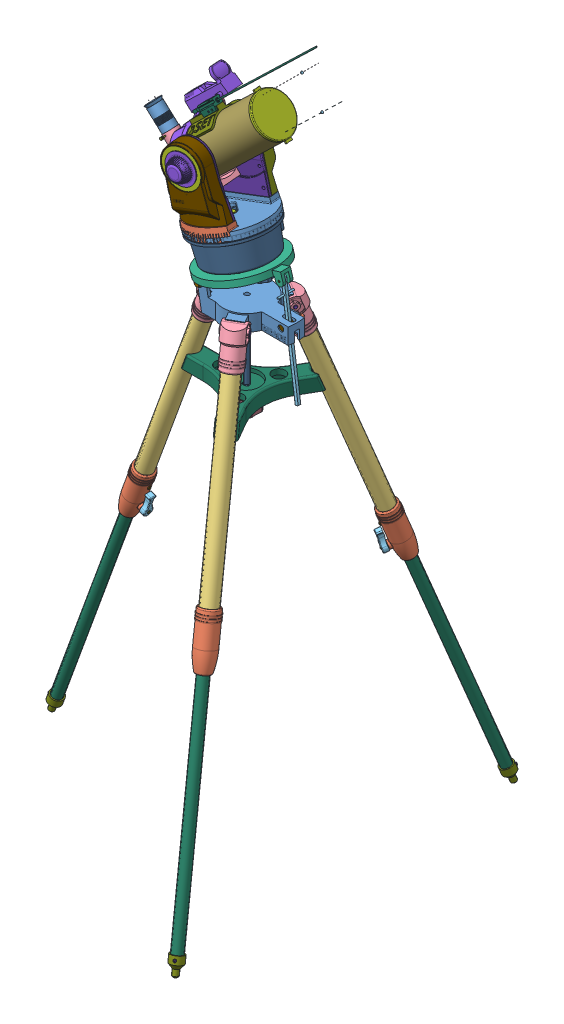
SolidWorks assembly telescope assemblage, configuration Défaut. Lengths in mm.
Overall size (798.62 1786.17 885.88).
260 component instances, 126 part files, 44 mates.
Components (placement in the parent):
- plateforme trepied-1: plateforme trepied [Défaut] at (-10.3731 0 -20) x (0 0 1) z (0 1 0) size (184.28 220 78.5)
- tube superieur-1: tube superieur [Défaut] at (-282.0109 -548.273 -53.7859) x (0 0 -1) z (-0.939693 0.34202 0) size (56 647 70.31)
  - liaison tube-1: liaison tube [Défaut] at (-33.7859 -53.3876 0) size (49 123 52)
  - tube superieur-1: tube superieur [Défaut] at (-33.7859 -3.3876 0) x (1 0 0) z (0 -1 0) size (38 38 530)
  - liaison tube plaque-1: liaison tube plaque [Défaut] at (-33.7859 -483.3876 0) x (-1 0 0) z (0 0 1) size (54 94 52.5)
  - manette fixation pied-1: manette fixation pied [Défaut] at (-52.9516 19.4533 -40.9) x (-1 0 0) z (0 0 1) size (22 50 29.31)
    - manette fixation pied-1: manette fixation pied [Défaut] at (-19.1657 -10.1591 0) size (22 50 15.3)
    - vis M8 fixation pied-1: vis M8 fixation pied [Défaut] at (-19.1657 -10.1591 6.2) x (1 0 0) z (0 -1 0) size (11 21.7 11)
    - Vis cr f90 M4-1: Vis cr f90 M4 [Défaut] at (-19.1657 -10.1591 1.7) size (7.4 7.4 13.11)
  - VisChcM8 50-2: VisChcM8 50 [Défaut] at (-55.5859 -557.3876 0) x (0 0 -1) z (1 0 0) size (12.3 12.3 56)
  - Vis cr M5-1: Vis cr M5 [Défaut] at (-33.7859 -20.3876 -23.15) x (0 1 0) z (0 0 1) size (7.7 7.7 9.33)
  - Vis cr M5-2: Vis cr M5 [Défaut] at (-33.7859 -516.3876 -23.15) size (7.7 7.7 9.33)
- axe M12-1: axe M12 [Défaut] at (-10.3731 0 -20) x (-0.923728 0 0.383049) z (0 -1 0) size (12.15 12.3 255.78)
- rondelle 30-1: rondelle 30 [Défaut] at (-10.3731 -220.4136 -20) x (0.988696 0 0.149935) z (0 1 0) size (30 30 2.3)
- Ecrou hexagonal ISO 4032, M 12-1: Ecrou hexagonal ISO 4032, M 12 [Défaut] at (-10.3731 -29.8 -20) x (0.866025 0 0.5) z (-0.5 0 0.866025) size (20.78 10.8 18)
- ecrou plastic M12-1: ecrou plastic M12 [Défaut] at (-21.7775 -251.8636 -36.5397) x (-0.587785 0 -0.809017) z (0 1 0) size (58 55.29 30.73)
  - ecrou plastic-1: ecrou plastic [Défaut] at (-20.0843 0.4954 0) size (58 55.29 30)
  - insert M12-1: insert M12 [Défaut] at (-20.0843 0.4954 14.3) size (16 16 17.46)
- pied-1: pied [Défaut] at (-281.8601 -547.9154 -17.129) x (0 0 1) z (-0.34202 -0.939693 0) size (30.8 33.14 626.85)
  - tube inferieur-1: tube inferieur [Défaut] at (-2.871 0.0194 0) size (25 25 600)
  - pied-1: pied [Défaut] at (-2.871 0.0194 582.85) x (1 0 0) z (0 -1 0) size (30.8 44 30.8)
  - Vis cr M4-1: Vis cr M4 [Défaut] at (-2.871 15.3194 591.85) x (0 0 -1) z (0 -1 0) size (6.7 6.7 12.44)
- pied-2: pied [Défaut] at (122.8841 -547.9154 -256.5501) x (-0.866025 0 -0.5) z (0.17101 -0.939693 -0.296198) size (30.8 33.14 626.85)
  - tube inferieur-1: tube inferieur [Défaut] at (-2.871 0.0194 0) size (25 25 600)
  - pied-1: pied [Défaut] at (-2.871 0.0194 582.85) x (1 0 0) z (0 -1 0) size (30.8 44 30.8)
  - Vis cr M4-1: Vis cr M4 [Défaut] at (-2.871 15.3194 591.85) x (0 0 -1) z (0 -1 0) size (6.7 6.7 12.44)
- pied-3: pied [Défaut] at (127.8567 -547.9154 213.6791) x (0.866025 0 -0.5) z (0.17101 -0.939693 0.296198) size (30.8 33.14 626.85)
  - tube inferieur-1: tube inferieur [Défaut] at (-2.871 0.0194 0) size (25 25 600)
  - pied-1: pied [Défaut] at (-2.871 0.0194 582.85) x (1 0 0) z (0 -1 0) size (30.8 44 30.8)
  - Vis cr M4-1: Vis cr M4 [Défaut] at (-2.871 15.3194 591.85) x (0 0 -1) z (0 -1 0) size (6.7 6.7 12.44)
- tube superieur-2: tube superieur [Défaut] at (154.7052 -548.273 -238.3523) x (0.866025 0 0.5) z (0.469846 0.34202 -0.813798) size (56 647 70.31)
  - liaison tube-1: liaison tube [Défaut] at (-33.7859 -53.3876 0) size (49 123 52)
  - tube superieur-1: tube superieur [Défaut] at (-33.7859 -3.3876 0) x (1 0 0) z (0 -1 0) size (38 38 530)
  - liaison tube plaque-1: liaison tube plaque [Défaut] at (-33.7859 -483.3876 0) x (-1 0 0) z (0 0 1) size (54 94 52.5)
  - manette fixation pied-1: manette fixation pied [Défaut] at (-52.9516 19.4533 -40.9) x (-1 0 0) z (0 0 1) size (22 50 29.31)
    - manette fixation pied-1: manette fixation pied [Défaut] at (-19.1657 -10.1591 0) size (22 50 15.3)
    - vis M8 fixation pied-1: vis M8 fixation pied [Défaut] at (-19.1657 -10.1591 6.2) x (1 0 0) z (0 -1 0) size (11 21.7 11)
    - Vis cr f90 M4-1: Vis cr f90 M4 [Défaut] at (-19.1657 -10.1591 1.7) size (7.4 7.4 13.11)
  - VisChcM8 50-2: VisChcM8 50 [Défaut] at (-55.5859 -557.3876 0) x (0 0 -1) z (1 0 0) size (12.3 12.3 56)
  - Vis cr M5-1: Vis cr M5 [Défaut] at (-33.7859 -20.3876 -23.15) x (0 1 0) z (0 0 1) size (7.7 7.7 9.33)
  - Vis cr M5-2: Vis cr M5 [Défaut] at (-33.7859 -516.3876 -23.15) size (7.7 7.7 9.33)
- tube superieur-3: tube superieur [Défaut] at (96.1863 -548.273 232.1382) x (-0.866025 0 0.5) z (0.469846 0.34202 0.813798) size (56 647 70.31)
  - liaison tube-1: liaison tube [Défaut] at (-33.7859 -53.3876 0) size (49 123 52)
  - tube superieur-1: tube superieur [Défaut] at (-33.7859 -3.3876 0) x (1 0 0) z (0 -1 0) size (38 38 530)
  - liaison tube plaque-1: liaison tube plaque [Défaut] at (-33.7859 -483.3876 0) x (-1 0 0) z (0 0 1) size (54 94 52.5)
  - manette fixation pied-1: manette fixation pied [Défaut] at (-52.9516 19.4533 -40.9) x (-1 0 0) z (0 0 1) size (22 50 29.31)
    - manette fixation pied-1: manette fixation pied [Défaut] at (-19.1657 -10.1591 0) size (22 50 15.3)
    - vis M8 fixation pied-1: vis M8 fixation pied [Défaut] at (-19.1657 -10.1591 6.2) x (1 0 0) z (0 -1 0) size (11 21.7 11)
    - Vis cr f90 M4-1: Vis cr f90 M4 [Défaut] at (-19.1657 -10.1591 1.7) size (7.4 7.4 13.11)
  - VisChcM8 50-2: VisChcM8 50 [Défaut] at (-55.5859 -557.3876 0) x (0 0 -1) z (1 0 0) size (12.3 12.3 56)
  - Vis cr M5-1: Vis cr M5 [Défaut] at (-33.7859 -20.3876 -23.15) x (0 1 0) z (0 0 1) size (7.7 7.7 9.33)
  - Vis cr M5-2: Vis cr M5 [Défaut] at (-33.7859 -516.3876 -23.15) size (7.7 7.7 9.33)
- axe reglage altitude-1: axe reglage altitude [Défaut] at (94.0034 -12 -20) x (0.990738 0.135788 0) z (0 0 -1) size (14 14 35)
- VisM8 15 reglage montage equatorial-1: VisM8 15 reglage montage equatorial [Défaut] at (69.6004 -12.4568 -44.1703) x (-0.999825 -0.018716 0) z (0.018716 -0.999825 0) size (48.14 28.09 16.29)
  - languette-1: languette [Défaut] at (-24.4073 4.8297 0) size (45 10 2.8)
  - VisM8 15 reglage montage equatorial-1: VisM8 15 reglage montage equatorial [Défaut] at (-24.4073 -3.1703 0) x (0 0 1) z (0 -1 0) size (12 12 28.09)
  - CHCM3-10-1: CHCM3-10 [Défaut] at (-24.4073 4.8297 6.5) x (-1 0 0) z (0 0 -1) size (5 5 12.5)
  - rondelle 16-1: rondelle 16 [Défaut] at (-24.4073 -3.1703 0) x (0.999837 0 -0.018032) z (0 -1 0) size (16 16 1)
- regle-1: regle [Défaut] at (116.2056 -173.9924 -20) x (0 0 1) z (-0.135788 0.990738 0) size (40 8.8 260)
- plateau inclinable-1: plateau inclinable [Défaut] at (2.5363 78.221 -20) x (0.956126 0.292954 0) z (0.292954 -0.956126 0) size (206.4 185 50.37)
  - plateau inclinable-1: plateau inclinable [Défaut] at (-28.5 -0.1435 0) size (206.4 185 37.6)
  - Vis  M6-24-1: Vis  M6-24 [Défaut] at (75.7 -11.9435 22.75) x (-1 0 0) z (0 1 0) size (6 6 24)
  - rondelle 16-7: rondelle 16 [Défaut] at (-81.5 62.9965 28.6) x (-0.476926 0 0.878943) z (0 1 0) size (16 16 1)
  - rondelle 16-8: rondelle 16 [Défaut] at (-81.5 48 28.6) x (-0.476926 0 0.878943) z (0 1 0) size (16 16 1)
  - rondelle 16-9: rondelle 16 [Défaut] at (-81.5 56 28.6) x (-0.476926 0 0.878943) z (0 1 0) size (16 16 1)
  - rondelle 16-10: rondelle 16 [Défaut] at (-81.5 -56.2835 28.6) x (0.476926 0 -0.878943) z (0 -1 0) size (16 16 1)
  - rondelle 16-11: rondelle 16 [Défaut] at (-81.5 -48 28.6) x (0.476926 0 -0.878943) z (0 -1 0) size (16 16 1)
  - rondelle 16-12: rondelle 16 [Défaut] at (-81.5 -63.2835 28.6) x (0.476926 0 -0.878943) z (0 -1 0) size (16 16 1)
  - EcrouH8 nylstop-1: EcrouH8 nylstop [Défaut] at (-81.5 -48 28.6) x (0 0 -1) z (0 -1 0) size (13 15.01 7.1)
  - EcrouH8 nylstop-2: EcrouH8 nylstop [Défaut] at (-81.5 48 28.6) x (0 0 1) z (0 1 0) size (13 15.01 7.1)
  - VisHm8_25-1: VisHm8_25 [Défaut] at (-81.5 -64.2835 28.6) x (0.866025 0 0.5) z (0 1 0) size (13 15.01 29.5)
  - VisHm8_25-2: VisHm8_25 [Défaut] at (-81.5 63.9965 28.6) x (-0.866025 0 -0.5) z (0 -1 0) size (13 15.01 29.5)
  - vis plastique M6-1: vis plastique M6 [Défaut] at (-89.0406 -5.4634 33.1) x (-0.885007 -0.465577 0) z (0 0 -1) size (33.9 32.72 44.02)
    - bouton plastic-1: bouton plastic [Défaut] at (-10.2565 0.6155 0) size (33.9 32.72 15)
    - Vis  M6 30-1: Vis  M6 30 [Défaut] at (-10.2565 0.6155 15) x (-0.5 0.866025 0) z (0 0 1) size (10 11.55 34.02)
    - rondelle 12-1: rondelle 12 [Défaut] at (-10.2565 0.6155 32.1) size (11.9 11.9 1)
    - Truac-1: Truac [Défaut] at (-10.2565 0.6155 33.1) x (0 0 1) z (-0.309017 0.951057 0) size (0.6 8.54 9)
    - Ressort de compression, 9x0,4-1: Ressort de compression, 9x0,4 [Défaut] at (-10.2565 0.6155 32.1) x (0 0 -1) z (0.885007 0.465577 0) size (11.52 9.7 9.88)
  - vis plastique M6-2: vis plastique M6 [Défaut] at (14.4594 -5.4634 33.1) x (-0.885007 -0.465577 0) z (0 0 -1) size (33.9 32.72 44.02)
    - bouton plastic-1: bouton plastic [Défaut] at (-10.2565 0.6155 0) size (33.9 32.72 15)
    - Vis  M6 30-1: Vis  M6 30 [Défaut] at (-10.2565 0.6155 15) x (-0.5 0.866025 0) z (0 0 1) size (10 11.55 34.02)
    - rondelle 12-1: rondelle 12 [Défaut] at (-10.2565 0.6155 32.1) size (11.9 11.9 1)
    - Truac-1: Truac [Défaut] at (-10.2565 0.6155 33.1) x (0 0 1) z (-0.309017 0.951057 0) size (0.6 8.54 9)
    - Ressort de compression, 9x0,4-1: Ressort de compression, 9x0,4 [Défaut] at (-10.2565 0.6155 32.1) x (0 0 -1) z (0.885007 0.465577 0) size (11.52 9.7 9.88)
- cale-1: cale [Défaut] at (-13.285 -219.2636 -20) x (0 0 1) z (0 1 0) size (261.88 228.05 35)
- meade-1: meade [Défaut] at (-48.2669 146.7444 -20.1435) x (-0.956126 -0.292954 0) z (0 0 -1) size (480.47 493.64 231.58)
  - fourche-1: fourche [Défaut] at (-637.6539 13.0791 484.13) x (0.045417 -0.017413 0.998816) z (-0.998966 0.001172 0.045444) size (198.85 238.33 188.61)
    - branche equilibrage-1: branche equilibrage [Défaut] at (-444.0293 45.9192 -837.0232) x (0.999848 0.017413 0.00001) z (0.00001 -0.001172 0.999999) size (42.16 177.75 110.07)
    - Plaque carter équilibrage-1: Plaque carter équilibrage [Défaut] at (-443.0317 45.9366 -837.0903) x (0.999848 0.017413 0.00001) z (0.00001 -0.001172 0.999999) size (27.56 165.18 109.18)
    - Plaque carter équilibrage-2: Plaque carter équilibrage [Défaut] at (-468.0617 45.0668 -480.7137) x (-0.999848 -0.017413 -0.00001) z (-0.00001 0.001172 -0.999999) size (27.56 165.18 109.18)
    - branche motorisée-1: branche motorisée [Défaut] at (-441.716 45.9434 -837.1795) x (0.999848 0.017413 0.00001) z (0.00001 -0.001172 0.999999) size (49.59 177.72 110.04)
    - PIED DE fourche-1: PIED DE fourche [Défaut] at (-454.4692 -14.4541 -658.8869) x (0.999848 0.017413 0.00001) z (0.00001 -0.001172 0.999999) size (191.94 35.1 188.57)
      - Pied de fourche-1: Pied de fourche [Défaut] at (12.1809 59.9857 -178.2534) size (191.94 35.1 188.57)
      - Pied de fourche1-1: Pied de fourche1 [Défaut] at (-12.1809 59.9857 178.0188) x (-1 0 0) z (0 0 -1) size (54.8 35.1 115.86)
    - rondelle vis m8_50-1: rondelle vis m8_50 [Défaut] at (-454.2843 -25.0712 -659.0167) x (0.997592 0.017452 -0.067129) z (0.017413 -0.999848 -0.001172) size (26.8 26.16 7)
    - VisHM8_50-1: VisHM8_50 [Défaut] at (-454.3818 -19.4721 -659.0102) x (0.997592 0.017452 -0.067129) z (0.017413 -0.999848 -0.001172) size (12.6 14.55 55.47)
    - limiteur de couple embase-1: limiteur de couple embase [Défaut] at (-453.5008 -70.0544 -659.0694) x (0.06714 0 0.997744) z (-0.997592 -0.017452 0.067129) size (25.3 5 25.3)
    - Roue à denture hélicoïdale m=0,5 Z=60-1: Roue à denture hélicoïdale m=0,5 Z=60 [Défaut] at (-453.6431 -61.8856 -659.0599) x (0.201032 0.002353 0.979582) z (-0.017413 0.999848 0.001172) size (31.07 31.07 6.34)
    - Levier de débrayage-1: Levier de débrayage [Défaut] at (-491.4971 43.1006 -833.8173) x (0.963244 0.01709 -0.268082) z (0.268062 0.003539 0.963395) size (36.12 10 38.96)
    - plateau-1: plateau [Défaut] at (-454.3861 -19.2221 -659.0099) x (-0.997592 -0.017452 0.067129) z (0.017413 -0.999848 -0.001172) size (170 170 47)
    - EcrouHM 20-2: EcrouHM 20 [Défaut] at (-453.9456 -44.5183 -659.0395) x (0.06714 0 0.997744) z (-0.017413 0.999848 0.001172) size (30 34.64 12)
    - motoreducteur fourche-1: motoreducteur fourche [Défaut] at (-542.1299 45.8782 -641.824) x (0.06714 0 0.997744) z (0.997592 0.017452 -0.067129) size (70.5 139.71 33.06)
      - rep. 01 pignon arbre moteur + disque-1: rep. 01 pignon arbre moteur + disque [Défaut] at (0 -0.36 0) size (19 10.8 19)
      - rep. 02-03 roue Z56-1: rep. 02-03 roue Z56 [Défaut] at (0.8779 -0.6486 0.8082) x (0.995701 0 0.092628) z (-0.092628 0 0.995701) size (28.76 10.95 28.76)
      - rep. 08-09 roue inter-1: rep. 08-09 roue inter [Défaut] at (-0.15 -0.2381 0) x (1 0 0) z (0 0 1) size (12.96 5.74 12.96)
      - rep. 06-07 roue inter-1: rep. 06-07 roue inter [Défaut] at (-0.15 -0.0981 0) x (1 0 0) z (0 0 1) size (13 5.74 13)
      - rep. 04-05 roue inter-1: rep. 04-05 roue inter [Défaut] at (-21.6079 -0.6386 5.1059) x (0.907401 0 -0.420265) z (0.420265 0 0.907401) size (13 5.74 13)
      - bati-1: bati [Défaut] at (103.3128 129.885 -87.3106) size (70.5 138.91 24)
        - Axe Rep19bis-1: Axe Rep19bis [Défaut] at (-92.1856 -130.245 98.2871) x (-0.137137 0 0.990552) z (-0.990552 0 -0.137137) size (3 14 3)
        - moteur-1: moteur [Défaut] at (-103.3128 -129.885 87.3106) size (18 46.5 24)
        - axe-1: axe [Défaut] at (-111.605 -120.0821 97.7106) x (0.934599 0 -0.355704) z (0 -1 0) size (3 3 39)
        - bati2-1: bati2 [Défaut] at (-77.4849 -277.8736 138.6581) x (1 0 0) z (0 0 -1) size (17.4 55.11 17.4)
          - rondelle alu-1: rondelle alu [Défaut] at (-55.9783 -35.2009 30.6529) size (17.4 2.5 17.4)
          - Rondelle M6_1-1: Rondelle M6_1 [Défaut] at (-55.9783 -35.2009 30.6529) size (16.67 2.55 16.67)
          - rondelle alu_1-1: rondelle alu_1 [Défaut] at (-55.9783 -35.2009 30.6529) size (17.4 2.5 17.4)
          - Entretoise_1-1: Entretoise_1 [Défaut] at (-55.9783 -35.2009 30.6529) size (16.5 6 16.5)
          - Entretoise-1: Entretoise [Défaut] at (-55.9783 -35.2009 30.6529) size (16.5 6 16.5)
          - Rondelle M6-1: Rondelle M6 [Défaut] at (-55.9783 -35.2009 30.6529) size (16.67 2.55 16.67)
          - rep. 16 Ecrou M6-1: rep. 16 Ecrou M6 [Défaut] at (18.5294 -120.4752 48.0628) x (-0.896454 0 -0.443136) z (-0.443136 0 0.896454) size (12.68 6 11.39)
        - corps1-1: corps1 [Défaut] at (-126.5989 -147.7633 97.7106) size (62.7 74.5 12)
        - corps2-1: corps2 [Défaut] at (-126.5989 -147.7633 85.7106) size (62.7 50 12) (hidden)
        - châpe en alu-1: châpe en alu [Défaut] at (-133.4632 -157.3984 87.2051) size (33.3 38 19.61)
      - vis-1: vis [Défaut] at (7.3554 -71.4832 9.6533) x (1 0 0) z (0 1 0) size (33.09 33.06 82.71)
        - Vis san fin m=0,5 - 1 filet(s)-2: Vis san fin m=0,5 - 1 filet(s) [Défaut] at (-0.6479 -0.6412 0.3804) x (0.7262 -0.687484 0) z (0 0 1) size (8.16 8.16 68.9)
        - rep12-4: rep12 [Défaut] at (-11.6724 36.0347 43.7266) x (0.537117 -0.843508 0) z (-0.843508 -0.537117 0) size (23.91 29.81 24)
      - engrenage-1: engrenage [Défaut] at (-45.9983 -125.8694 31.0757) x (-0.919401 0 0.393321) z (0.393321 0 0.919401) size (12.99 17.44 12.99)
        - rep.11SLDPRT-1: rep.11SLDPRT [Défaut] at (-64.557 -106.8565 -14.5787) size (9.52 16 9.52)
        - rep. yacine-1: rep. yacine [Défaut] at (-64.557 -106.8565 -14.5787) size (12.99 1.44 12.99)
      - Vis à tête cylindrique à six pans creux Chc M2,5 - 8-1: Vis à tête cylindrique à six pans creux Chc M2,5 - 8 [Défaut] at (6.7074 -20.6971 10.2945) x (0.636786 0 0.771041) z (0 -1 0) size (4.2 4.2 10.57)
      - joint 9 5 emb-1: joint 9 5 emb [Défaut] at (6.7074 -89.1506 10.2945) size (13.5 2 13.5)
      - joint 9 5 emb-2: joint 9 5 emb [Défaut] at (6.7074 -53.1506 10.2945) size (13.5 2 13.5)
    - Vis sans tête à six pans creux à bout cuvette M3 - 3-1: Vis sans tête à six pans creux à bout cuvette M3 - 3 [Réaliste] at (-445.1418 -17.1499 -659.6319) x (-0.019293 -0.859815 -0.51024) z (0.066624 -0.510307 0.857408) size (3.03 3.08 3.04)
    - Vis à tête cylindrique bombée cruciforme type H M3 - 10-1: Vis à tête cylindrique bombée cruciforme type H M3 - 10 [Filetage Réaliste] at (-521.841 56.7793 -695.504) x (-0.997592 -0.017452 0.067129) z (-0.0364 0.955572 -0.292501) size (12.58 5.6 5.6)
    - Vis à tête cylindrique bombée cruciforme type H M3 - 10-2: Vis à tête cylindrique bombée cruciforme type H M3 - 10 [Filetage Réaliste] at (-508.9533 16.8988 -611.179) x (-0.997592 -0.017452 0.067129) z (-0.040277 -0.642181 -0.765494) size (12.58 5.6 5.6)
    - Vis à tête cylindrique bombée cruciforme type H M3 - 10-3: Vis à tête cylindrique bombée cruciforme type H M3 - 10 [Filetage Réaliste] at (-514.8616 16.8988 -698.9804) x (-0.997592 -0.017452 0.067129) z (-0.068087 0.06176 -0.995766) size (12.58 5.6 5.6)
    - Vis à tête cylindrique bombée cruciforme type H M3 - 10-4: Vis à tête cylindrique bombée cruciforme type H M3 - 10 [Filetage Réaliste] at (-521.2936 154.7556 -654.4481) x (-0.997592 -0.017452 0.067129) z (-0.06714 0 -0.997744) size (12.58 5.6 5.6)
    - Vis à tête cylindrique bombée cruciforme type H M3 - 10-5: Vis à tête cylindrique bombée cruciforme type H M3 - 10 [Filetage Réaliste] at (-516.3356 56.7793 -613.689) x (-0.997592 -0.017452 0.067129) z (-0.06714 0 -0.997744) size (12.58 5.6 5.6)
    - Vis à tête cylindrique bombée cruciforme type H M3 - 10-7: Vis à tête cylindrique bombée cruciforme type H M3 - 10 [Filetage Réaliste] at (-393.6444 157.0051 -663.0973) x (0.997592 0.017452 -0.067129) z (0.06714 0 0.997744) size (12.58 5.6 5.6)
    - Vis à tête cylindrique bombée cruciforme type H M3 - 10-8: Vis à tête cylindrique bombée cruciforme type H M3 - 10 [Filetage Réaliste] at (-401.1787 18.9039 -706.6898) x (0.997592 0.017452 -0.067129) z (0.06714 0 0.997744) size (12.58 5.6 5.6)
    - Vis à tête cylindrique bombée cruciforme type H M3 - 10-10: Vis à tête cylindrique bombée cruciforme type H M3 - 10 [Filetage Réaliste] at (-395.1895 59.0113 -704.086) x (0.997592 0.017452 -0.067129) z (0.06714 0 0.997744) size (12.58 5.6 5.6)
    - Vis à tête cylindrique fendue CS M4 - 10-1: Vis à tête cylindrique fendue CS M4 - 10 [Défaut] at (-539.7157 125.5672 -628.3483) x (0.067415 -0.016315 0.997592) z (-0.997592 -0.017452 0.067129) size (7 7 10.62)
    - Vis à tête cylindrique fendue CS M4 - 10-2: Vis à tête cylindrique fendue CS M4 - 10 [Défaut] at (-538.2089 116.0774 -615.8713) x (0.067415 -0.016315 0.997592) z (-0.997592 -0.017452 0.067129) size (7 7 10.62)
    - Vis à tête cylindrique fendue CS M4 - 10-3: Vis à tête cylindrique fendue CS M4 - 10 [Défaut] at (-539.3849 106.5701 -628.3705) x (0.067415 -0.016315 0.997592) z (-0.997592 -0.017452 0.067129) size (7 7 10.62)
    - Vis à tête cylindrique bombée cruciforme type H M3 - 12-2: Vis à tête cylindrique bombée cruciforme type H M3 - 12 [Filetage Réaliste] at (-395.2704 18.9039 -618.8883) x (0.997592 0.017452 -0.067129) z (0.067129 0.000586 0.997744) size (14.59 5.6 5.6)
    - Vis à tête cylindrique bombée cruciforme type H M3 - 12-3: Vis à tête cylindrique bombée cruciforme type H M3 - 12 [Filetage Réaliste] at (-389.684 59.0113 -622.271) x (0.997592 0.017452 -0.067129) z (0.068185 -0.42423 0.902984) size (14.59 5.6 5.6)
    - Vis à tête cylindrique bombée cruciforme type H M3 - 25-1: Vis à tête cylindrique bombée cruciforme type H M3 - 25 [Filetage Réaliste] at (-516.5693 58.6063 -628.1014) x (-0.997592 -0.017452 0.067129) z (-0.067129 0.486457 -0.871122) size (32.61 5.6 5.6)
    - Vis à tête cylindrique bombée cruciforme type H M3 - 25-2: Vis à tête cylindrique bombée cruciforme type H M3 - 25 [Filetage Réaliste] at (-520.3322 72.7741 -680.3366) x (-0.997592 -0.017452 0.067129) z (-0.067129 0.486457 -0.871122) size (32.61 5.6 5.6)
    - Vis à tête cylindrique bombée cruciforme type H M3 - 25-3: Vis à tête cylindrique bombée cruciforme type H M3 - 25 [Filetage Réaliste] at (-519.8272 43.7786 -680.3706) x (-0.997592 -0.017452 0.067129) z (0.067053 0.00493 0.997737) size (32.61 5.6 5.6)
    - Vis à tête cylindrique bombée cruciforme type H M3 - 20-1: Vis à tête cylindrique bombée cruciforme type H M3 - 20 [Filetage Réaliste] at (-531.1265 -25.9655 -653.8459) x (-0.017413 0.999848 0.001172) z (0.998816 0.017342 0.045444) size (22.61 5.6 5.6)
    - Vis à tête cylindrique bombée cruciforme type H M3 - 20-2: Vis à tête cylindrique bombée cruciforme type H M3 - 20 [Filetage Réaliste] at (-512.8439 -25.695 -612.9812) x (-0.017413 0.999848 0.001172) z (0.998816 0.017342 0.045444) size (22.61 5.6 5.6)
    - Vis à tête cylindrique bombée cruciforme type H M3 - 20-3: Vis à tête cylindrique bombée cruciforme type H M3 - 20 [Filetage Réaliste] at (-517.7505 -25.6821 -696.841) x (-0.017413 0.999848 0.001172) z (0.998816 0.017342 0.045444) size (22.61 5.6 5.6)
    - Vis à tête cylindrique bombée cruciforme type H M3 - 20-4: Vis à tête cylindrique bombée cruciforme type H M3 - 20 [Filetage Réaliste] at (-395.7403 -23.5476 -705.0512) x (-0.017413 0.999848 0.001172) z (0.998816 0.017342 0.045444) size (22.61 5.6 5.6)
    - Vis à tête cylindrique bombée cruciforme type H M3 - 20-5: Vis à tête cylindrique bombée cruciforme type H M3 - 20 [Filetage Réaliste] at (-377.4577 -23.2771 -664.1865) x (-0.017413 0.999848 0.001172) z (0.998816 0.017342 0.045444) size (22.61 5.6 5.6)
    - Vis à tête cylindrique bombée cruciforme type H M3 - 20-6: Vis à tête cylindrique bombée cruciforme type H M3 - 20 [Filetage Réaliste] at (-390.8337 -23.5604 -621.1914) x (-0.017413 0.999848 0.001172) z (0.998816 0.017342 0.045444) size (22.61 5.6 5.6)
  - tube-1: tube [Défaut] at (-30.0954 77.7985 3.4044) x (0.112402 0 0.993663) z (-0.888013 0.448711 0.100451) size (229.47 195.18 484.9)
    - Capuchon port photo-2: Capuchon port photo [Défaut] at (20.0265 52.1414 -183.8549) x (0.753442 -0.654583 0.06202) z (-0.29492 -0.252137 0.921656) size (39.95 39.82 23.78)
    - support objectif-2: support objectif [Défaut] at (0 67.5 -76) size (179.88 130.77 134.7)
    - Palier d'embrayage-2: Palier d'embrayage [Défaut] at (24.7034 252.6163 -72.3954) x (0.997744 -0.06714 0) z (-0.06714 -0.997744 0) size (14.91 34.8 28.76)
    - palier-2: palier [Défaut] at (-93.6662 67.5 0) x (1 0 0) z (0 -0.589029 0.808112) size (10.05 25.5 25.5)
    - Roue à denture hélicoïdale m=0,5 Z=60-3: Roue à denture hélicoïdale m=0,5 Z=60 [Défaut] at (-77.15 67.5 0) x (0 0.783284 -0.621664) z (1 0 0) size (31.07 31.07 6.34)
    - Plaque repérage angulaire-3: Plaque repérage angulaire [Défaut] at (-159.1429 162.8547 -174.0321) x (0.997744 -0.051519 0.043053) z (-0.06714 -0.765605 0.639798) size (6.77 89 88.85)
    - molette blocage vertical-2: molette blocage vertical [Défaut] at (25.2373 156.4775 -169.1848) x (0.997744 -0.051429 0.043161) z (-0.06714 -0.764265 0.641398) size (31.87 70 69.98)
    - molette blocage 2 vertical-2: molette blocage 2 vertical [Défaut] at (-32.8172 155.1442 169.8822) x (-0.997741 -0.051084 -0.043619) z (0.067172 -0.759198 -0.647384) size (27.85 70 69.98)
    - Plaque repérage angulaire-4: Plaque repérage angulaire [Défaut] at (151.5627 161.1167 174.9858) x (-0.997741 -0.051084 -0.043619) z (0.067172 -0.759198 -0.647384) size (6.77 89 88.85)
    - Embout fileté-2: Embout fileté [Défaut] at (31.1097 71.2083 -217.7977) x (0.995668 0.069272 0.06202) z (-0.030498 -0.386808 0.921656) size (96.08 90.33 41.21)
    - miroir-2: miroir [Défaut] at (1.5401 49.2079 -414.2886) x (0 -0.998075 0.06202) z (-0.383759 0.057271 0.921656) size (89.51 86.43 44.67)
    - tube-2: tube [Défaut] at (0 67.5 -53.7618) x (0 0 -1) z (1 0 0) size (225 100 100)
    - menisque-2: menisque [Défaut] at (-10.827 126.3859 145.8849) x (-0.376431 0.924349 0.062271) z (0.377105 0.091483 0.921641) size (110.67 106.16 46.27)
      - menisque-1: menisque [Défaut] at (-56.116 -127.6725 -342.9742) size (27.57 28.77 19.69)
      - Piece1-1: Piece1 [Défaut] at (-57.8098 16.1933 3.3103) x (0.972599 -0.230535 0.030091) z (-0.028457 0.010411 0.999541) size (92 86.87 40.19)
    - molette-2: molette [Défaut] at (16.1783 77.4199 -201.1536) x (0.997152 -0.042906 0.06202) z (-0.073715 -0.380942 0.921656) size (12.27 29.01 54.01)
    - Vis porte oculaire-2: Vis porte oculaire [Défaut] at (70.5773 71.9334 3.0696) x (0.833291 0.517003 -0.195792) z (-0.515568 0.854579 0.062325) size (15.46 8.19 13.39)
    - bouton miroir-3: bouton miroir [Défaut] at (118.3372 40.7094 -82.3) x (0.999979 -0.006557 0) z (0 0 1) size (83.58 43.34 43.14)
      - bouton miroir-1: bouton miroir [Défaut] at (-90.8002 18.3233 -120.2299) x (0.996615 -0.012919 0.081184) z (-0.081184 -0.309873 0.947306) size (41.27 12.61 13.28)
      - bouton miroir-2: bouton miroir [Défaut] at (-145.9581 -6.2943 -120.2299) x (-0.996615 0.012919 0.081184) z (0.081184 0.309873 0.947306) size (41.27 12.61 13.28)
      - petit miroir-1: petit miroir [Défaut] at (-118.5103 26.0141 2.75) x (0.999979 0.006557 0) z (0.004637 -0.707092 0.707107) size (30 26.01 35)
    - oculaire-2: oculaire [Défaut] at (0 149.5136 -0.7045) x (0 0 1) z (-1 0 0) size (38 81.5 38)
      - oculaire-1: oculaire [Défaut] at (-78.8455 -41.743 0) size (38 81.5 38)
      - lentille-1: lentille [Défaut] at (-81.1151 5.0064 0) x (0 -1 0) z (0 0 1) size (10.53 25 25)
        - lentille 1-1: lentille 1 [Défaut] at (-6.7507 2.2696 0) size (8.01 25 25)
        - lentille 2-1: lentille 2 [Défaut] at (-12.7507 2.2696 0) size (4.52 25 25)
      - lentille-2: lentille [Défaut] at (-76.963 10.0077 1.2678) x (0 1 0) z (-0.558618 0 0.829425) size (10.53 25 25)
        - lentille 1-1: lentille 1 [Défaut] at (-6.7507 2.2696 0) size (8.01 25 25)
        - lentille 2-1: lentille 2 [Défaut] at (-12.7507 2.2696 0) size (4.52 25 25)
    - faisceau2-2: faisceau2 [Défaut] at (0 78.827 -14.9477) x (0 0 -1) z (1 0 0) size (437.42 120.49 0.34)
    - fleche-13: fleche [Défaut] at (0 108.7031 110.8339) x (0 0 1) z (-0.886861 -0.462037 0) size (8 5.6 5.6)
    - fleche-14: fleche [Défaut] at (0 88.228 83.446) x (0 0.178036 -0.984024) z (1 -0.000403 -0.000073) size (8 5.6 5.6)
    - fleche-15: fleche [Défaut] at (0 75.6322 94.3005) x (0 0.005533 0.999985) z (0.072331 0.997365 -0.005519) size (8 5.6 5.6)
    - fleche-16: fleche [Défaut] at (0 108.7103 294.2676) x (0 0.017452 0.999848) z (-0.523715 0.851763 -0.014868) size (8 5.6 5.6)
    - fleche-17: fleche [Défaut] at (0 127.4306 -74.061) x (0 -0.974863 -0.222804) z (-0.735553 0.150943 -0.660438) size (8 5.6 5.6)
    - fleche-18: fleche [Défaut] at (0 183.519 -69.8214) x (0 -1 0) z (-0.316126 0 0.948717) size (8 5.6 5.6)
    - faisceau1-2: faisceau1 [Défaut] at (0 -20.7845 -6.8996) x (0 0 -1) z (1 0 0) size (447.26 167.74 0.41)
    - fleche-19: fleche [Défaut] at (0 30.6251 284.852) x (0 0 1) z (-0.426184 0.904636 0) size (8 5.6 5.6)
    - fleche-20: fleche [Défaut] at (0 27.6512 105.4051) x (0 0 1) z (-0.740163 -0.672427 0) size (8 5.6 5.6)
    - fleche-21: fleche [Défaut] at (0 46.7601 79.6116) x (0 -0.171906 -0.985113) z (0.984293 0.173915 -0.030349) size (8 5.6 5.6)
    - fleche-22: fleche [Défaut] at (0 59.5724 94.0494) x (0 -0.005145 0.999987) z (-0.101559 -0.994816 -0.005119) size (8 5.6 5.6)
    - fleche-23: fleche [Défaut] at (0 127.1897 -84.7907) x (0 -0.982309 0.187268) z (-0.405585 0.171174 0.897887) size (8 5.6 5.6)
    - fleche-24: fleche [Défaut] at (0 183.4575 -88.3366) x (0 -1 0) z (-0.976187 0 0.216931) size (8 5.6 5.6)
    - cache-2: cache [Défaut] at (0 67.5 174.5) x (0 0 -1) z (1 0 0) size (10 111 100)
    - Module LNT-2: Module LNT [Défaut] at (0 67.5 -16) x (0.999806 -0.019718 0) z (0 0 1) size (140.9 99.11 110)
    - Vis à tête cylindrique fendue CS M3 - 10-1: Vis à tête cylindrique fendue CS M3 - 10 [Défaut] at (27 106.7707 -61.5) size (5.5 5.5 12.01)
    - Pièce1^tube-1: Pièce1^tube [Défaut] at origin (virtual)
  - CARTER EMBASE-2: CARTER EMBASE [Défaut] at (-38.5593 -33.7526 0) x (-1 0 0) z (0 0 -1) size (208.81 81 208.82)
    - Carter embase-1: Carter embase [Défaut] at (-38.5593 34.3526 0) size (182.1 77.5 182)
    - palier-1: palier [Défaut] at (-38.7022 18.1339 0.128) x (-0.744983 0 0.667084) z (0.667084 0 0.744983) size (45.68 15.3 45.68)
      - palier alu-1: palier alu [Défaut] at (-0.1919 7.7813 0) size (40 13.5 40)
      - palier axial-1: palier axial [Défaut] at (-0.1919 -6.6187 0) size (33 6.3 33)
      - palier axial-2: palier axial [Défaut] at (-0.1919 8.6813 0) x (-0.837169 0 -0.546944) z (-0.546944 0 0.837169) size (33 6.3 33)
    - plaque branchement-1: plaque branchement [Défaut] at (-38.5593 -18.7385 -76.5024) x (1 0 0) z (0 0.068841 0.997628) size (62.31 43.19 20.2)
    - carter couvercle-1: carter couvercle [Défaut] at (-38.5593 -43.1474 0) x (0 0 1) z (-1 0 0) size (145 23 145)
    - anneau guide-1: anneau guide [Défaut] at (-38.5593 19.8526 0) x (-0.683843 0 0.729629) z (0 1 0) size (46.6 56.5 4.2)
    - support palier-1: support palier [Défaut] at (-38.5593 58.1532 0) x (0.258819 0 -0.965926) z (0.965926 0 0.258819) size (170.5 70.67 170.49)
    - reducteur embase-1: reducteur embase [Défaut] at (-74.9499 2.4826 -18.0358) x (0 0 1) z (0 -1 0) size (101.77 85.1 39.66)
      - rep. 01 pignon arbre moteur + disque-1: rep. 01 pignon arbre moteur + disque [Défaut] at (0.9543 -1.36 18.0797) x (0.78085 0 0.624719) z (-0.624719 0 0.78085) size (19 10.8 19)
      - rep. 02-03 roue Z56-1: rep. 02-03 roue Z56 [Défaut] at (-12.7174 -0.5 -2.1104) x (0.531735 0 -0.846911) z (0.846911 0 0.531735) size (28.76 10.95 28.76)
      - rep. 08-09 roue inter-1: rep. 08-09 roue inter [Défaut] at (-2.3943 -0.3381 0.4364) x (0.975998 0 -0.217777) z (0.217777 0 0.975998) size (12.96 5.74 12.96)
      - rep. 06-07 roue inter-1: rep. 06-07 roue inter [Défaut] at (-3.1771 0.3019 0.7148) x (0.955582 0 -0.294727) z (0.294727 0 0.955582) size (13 5.74 13)
      - roue rep 12 (petite folle)-1: roue rep 12 (petite folle) [Défaut] at (0.2679 -0.4 -0.3808) x (0.999222 0 0.039446) z (-0.039446 0 0.999222) size (13 3.24 13)
      - rep. 04-05 roue inter-1: rep. 04-05 roue inter [Défaut] at (2.2907 -0.16 -1.8606) x (0.977065 0 0.21294) z (-0.21294 0 0.977065) size (13 5.74 13)
      - bati emb-1: bati emb [Défaut] at (103.3128 129.885 -87.3106) size (101.77 84.35 25.96)
        - coque droite emb-1: coque droite emb [Défaut] at (-103.3128 -129.885 87.3106) size (93.29 54 12.58)
        - Axe Rep19bis emb-1: Axe Rep19bis emb [Défaut] at (-103.9752 -130.143 87.3656) x (0.998781 0 -0.049366) z (0.049366 0 0.998781) size (3 15.3 3)
        - Axe Rep20.bis emb-1: Axe Rep20.bis emb [Défaut] at (-97.8983 -130.0094 79.9317) x (0.927514 0 0.373788) z (-0.373788 0 0.927514) size (3 22 3)
        - coque gauche emb-1: coque gauche emb [Défaut] at (-103.3128 -129.885 87.3106) size (94.76 55 11.51)
        - axe emb-1: axe emb [Défaut] at (-111.605 -119.0221 97.7106) x (0.824702 0 -0.565567) z (0 -1 0) size (3 3 15)
        - Axe Rep19bis emb-2: Axe Rep19bis emb [Défaut] at (-101.4828 -129.945 90.8669) x (0.715658 0 -0.698451) z (0.698451 0 0.715658) size (3 15.3 3)
        - moteur-2: moteur [Défaut] at (-103.3128 -129.885 87.3106) size (18 46.5 24)
        - châpe en alu emb-2: châpe en alu emb [Défaut] at (-103.4628 -123.4884 87.3106) size (32 38 21)
        - Entretoise emb-3: Entretoise emb [Défaut] at (-100.6729 -123.5884 80.7498) x (0.982912 0 0.184074) z (-0.184074 0 0.982912) size (17.65 5.7 17.65)
        - rondelle alu emb-3: rondelle alu emb [Défaut] at (-90.9589 -123.8884 68.1548) x (0.821605 0 0.570058) z (-0.570058 0 0.821605) size (17.4 2.65 17.4)
        - rep. 16 Ecrou M6 emb-2: rep. 16 Ecrou M6 emb [Défaut] at (-102.7157 -122.485 84.9564) x (0.99792 0 0.06446) z (-0.06446 0 0.99792) size (12.68 6 11.39)
        - Rondelle M6 emb-2: Rondelle M6 emb [Défaut] at (-94.2052 -123.7384 71.161) x (0.88187 0 0.471493) z (-0.471493 0 0.88187) size (16 1.8 16)
        - joint 9 5 emb-3: joint 9 5 emb [Défaut] at (-66.605 -149.1255 97.7106) size (13.5 2 13.5)
        - joint 9 5 emb-4: joint 9 5 emb [Défaut] at (-66.605 -183.1255 97.7106) x (0.837169 0 0.546944) z (0.546944 0 -0.837169) size (13.5 2 13.5)
        - rondelle alu emb-4: rondelle alu emb [Défaut] at (-91.5165 -167.7384 68.6232) x (0.832295 0 0.554332) z (-0.554332 0 0.832295) size (17.4 2.65 17.4)
        - Entretoise emb-4: Entretoise emb [Défaut] at (-30.2975 -208.6627 109.115) x (-0.835834 0 -0.548983) z (-0.548983 0 0.835834) size (17.65 5.7 17.65)
        - Rondelle M6 emb-3: Rondelle M6 emb [Défaut] at (-29.9622 -208.5127 109.2274) x (-0.837169 0 -0.546944) z (-0.546944 0 0.837169) size (16 1.8 16)
        - Vis à tête cylindrique bombée cruciforme type H M3 - 12-1: Vis à tête cylindrique bombée cruciforme type H M3 - 12 [Filetage Réaliste] at (-110.205 -142.8221 109.7106) x (0 0 -1) z (1 0 0) size (14.59 5.6 5.6)
        - Vis à tête cylindrique bombée cruciforme type H M3 - 12-2: Vis à tête cylindrique bombée cruciforme type H M3 - 12 [Filetage Réaliste] at (-93.3519 -120.1721 111.5106) x (0 0 -1) z (-0.592827 0.80533 0) size (14.59 5.6 5.6)
      - vis emb-1: vis emb [Défaut] at (37.3558 -36.1406 9.7588) x (1 0 0) z (0 1 0) size (25.74 25.82 76.16)
        - Vis san fin m=0,5 - 1 filet(s) emb-1: Vis san fin m=0,5 - 1 filet(s) emb [Défaut] at (-0.6479 -0.6412 0) size (8.16 8.16 68.9)
        - rep12 emb-3: rep12 emb [Défaut] at (-38.2155 6.7975 36.7974) x (0.996839 0.079451 0) z (0.079451 -0.996839 0) size (23.91 23.8 24)
      - engrenage-1: engrenage [Défaut] at (64.1683 106.4565 3.5924) x (0.967334 0 -0.253504) z (0.253504 0 0.967334) size (12.99 17.44 12.99)
        - rep.11SLDPRT-1: rep.11SLDPRT [Défaut] at (-64.557 -106.8565 -14.5787) size (9.52 16 9.52)
        - rep. yacine-1: rep. yacine [Défaut] at (-64.557 -106.8565 -14.5787) size (12.99 1.44 12.99)
      - Vis à tête cylindrique à six pans creux Chc M2,5 - 8-1: Vis à tête cylindrique à six pans creux Chc M2,5 - 8 [Défaut] at (36.7078 7.7163 10.4) x (1 0 0) z (0 -1 0) size (4.2 4.2 10.57)
    - Vis à tête fraisée FS M5 - 16-1: Vis à tête fraisée FS M5 - 16 [Défaut] at (-102.5593 -40.456 0) x (-1 0 0) z (0 1 0) size (10.32 10.4 16)
    - Vis à tête fraisée FS M5 - 16-2: Vis à tête fraisée FS M5 - 16 [Défaut] at (-6.5593 -40.456 55.4256) x (0.5 0 0.866025) z (0 1 0) size (10.32 10.4 16)
    - Vis à tête fraisée FS M5 - 16-3: Vis à tête fraisée FS M5 - 16 [Défaut] at (-6.5593 -40.456 -55.4256) x (0.5 0 -0.866025) z (0 1 0) size (10.32 10.4 16)
    - Vis à tête cylindrique bombée cruciforme type H M3 - 12-1: Vis à tête cylindrique bombée cruciforme type H M3 - 12 [Filetage Réaliste] at (-58.5127 -18.1174 -56.178) x (0 1 0) z (0 0 1) size (14.59 5.6 5.6)
    - Vis à tête cylindrique bombée cruciforme type H M3 - 12-2: Vis à tête cylindrique bombée cruciforme type H M3 - 12 [Filetage Réaliste] at (-89.2627 -18.7174 28.322) x (0 1 0) z (0 0 1) size (14.59 5.6 5.6)
    - Vis à tête cylindrique fendue CS M4 - 10-1: Vis à tête cylindrique fendue CS M4 - 10 [Défaut] at (-38.4593 -1.6174 37.562) x (1 0 0) z (0 1 0) size (7 7 10.62)
    - Vis à tête cylindrique fendue CS M4 - 10-2: Vis à tête cylindrique fendue CS M4 - 10 [Défaut] at (-31.0593 -0.5174 24.912) x (1 0 0) z (0 1 0) size (7 7 10.62)
    - Vis à tête cylindrique fendue CS M4 - 10-3: Vis à tête cylindrique fendue CS M4 - 10 [Défaut] at (-45.8593 -0.5174 24.912) x (1 0 0) z (0 1 0) size (7 7 10.62)
- Assemblage-1: Assemblage [Défaut] at (-173.0424 256.0479 -21.998) x (-0.107471 -0.032929 -0.993663) z (0.717601 0.689172 -0.100451) size (97.88 77.16 430.86)
  - montage-1: montage [Défaut] at (-9.6589 23.8863 105) size (28.9 22.7 356)
    - Pièce1-1: Pièce1 [Défaut] at (12.4057 3.1256 40) x (-1 0 0) z (0 0 -1) size (5.42 14 40)
    - vis_M3_chc M20 26-1: vis_M3_chc M20 26 [Défaut] at (-16.0943 -5.8744 19) x (0 0 -1) z (1 0 0) size (4 4 28.5)
    - pointeur-2: pointeur [Défaut] at (-16.3943 3.1256 0) size (27.7 22.7 356)
  - telescope v10 SET-1: telescope v10 SET [Défaut] at (-11.6532 -41.4489 0) size (97.88 71.37 131.47)
Mates (geometry in assembly coordinates):
- Coïncidente1: coincident anti-aligned: plane of plateforme trepied-1; plane of tube superieur-1/liaison tube-1
- Coïncidente2: coincident: plane of plateforme trepied-1; axis of tube superieur-1/liaison tube plaque-1 through (-31.9917 -99.2932 -23) axis (1 0 0)
- Coaxiale2: concentric aligned: cylinder of plateforme trepied-1 through (-91.3731 -24.5 -2) axis (0 0 -1) radius 4; cylinder of tube superieur-1/VisChcM8 50-2 through (-91.3731 -24.5 1.8) axis (0 0 -1) radius 4
- Coïncidente4: coincident: plane of plateforme trepied-1 through (4.0083 -93.7932 -8) normal (0 0 1); line of tube superieur-1/liaison tube plaque-1 through (-31.9917 -97.3892 -7.7499) axis (1 0 0)
- Angle1: planar angle = 0.349066 rad aligned: axis of plateforme trepied-1 through (-13.9917 -19.2932 -5) axis (0 0 -1); axis of tube superieur-1/liaison tube plaque-1 through (-13.9917 -108.5017 -47.0526) axis (0 -0.34202 -0.939693)
- Coaxiale3: concentric aligned: cylinder of plateforme trepied-1 through (-10.3731 -19 -20) axis (0 -1 0) radius 5.1; cylinder of axe M12-1 through (-10.3731 0 -20) axis (0 -1 0) radius 6
- Coïncidente6: coincident aligned: plane of plateforme trepied-1 through (-10.3731 0 -20) normal (0 1 0); plane of axe M12-1 through (-10.3731 0 -20) normal (0 1 0)
- Coaxiale4: concentric anti-aligned: cylinder of axe M12-1 through (-10.3731 0 -20) axis (0 -1 0) radius 6; cylinder of Ecrou hexagonal ISO 4032, M 12-1 through (-10.3731 -27.4 -20) axis (0 1 0) radius 4.4845
- Coïncidente7: coincident anti-aligned: plane of plateforme trepied-1 through (-10.3731 -19 -20) normal (0 -1 0); plane of Ecrou hexagonal ISO 4032, M 12-1 through (-6.4894 -19 -17.7578) normal (0 1 0)
- Parallèle2: parallel aligned: plane of plateforme trepied-1 through (-70.3731 -40 -76) normal (-1 0 0); plane of Ecrou hexagonal ISO 4032, M 12-1 through (-19.3731 -19 -14.8038) normal (-1 0 0)
- Coaxiale5: concentric aligned: cylinder of axe M12-1 through (-10.3731 0 -20) axis (0 -1 0) radius 6; cylinder of rondelle 30-1 through (-10.3731 -219.2636 -20) axis (0 -1 0) radius 6.75
- Coaxiale6: concentric anti-aligned: cylinder of axe M12-1 through (-10.3731 0 -20) axis (0 -1 0) radius 6; cylinder of ecrou plastic M12-1/ecrou plastic-1 through (-10.3731 -251.8646 -20) axis (0 1 0) radius 12.5
- Coaxiale7: concentric anti-aligned: cylinder of tube superieur-1/tube superieur-1 through (-99.5816 -47.0526 -20) axis (-0.34202 -0.939693 0) radius 19; cylinder of pied-1/tube inferieur-1 through (-487.0904 -1111.7244 -20) axis (0.34202 0.939693 0) radius 12.5
- Distance1: distance = 70 mm anti-aligned: plane of pied-1/tube inferieur-1 through (-281.8783 -547.9088 -20) normal (0.34202 0.939693 0); plane of tube superieur-1/liaison tube-1 through (-305.8197 -613.6873 -36.5) normal (-0.34202 -0.939693 0)
- Angle2: planar angle = 0.349066 rad aligned: axis of tube superieur-1/liaison tube plaque-1 through (-99.5816 -47.0526 -20) axis (-0.34202 -0.939693 0); axis of axe M12-1 through (-10.3731 0 -20) axis (0 -1 0)
- Coaxiale8: concentric anti-aligned: cylinder of axe reglage altitude-1 through (94.0034 -12 -37.5) axis (0 0 1) radius 7; cylinder of VisM8 15 reglage montage equatorial-1/VisM8 15 reglage montage equatorial-1 through (94.0034 -12 -41) axis (0 0 -1) radius 6
- Coïncidente35: coincident anti-aligned: plane of plateforme trepied-1 through (112.0034 -40 -40) normal (0 0 -1); plane of VisM8 15 reglage montage equatorial-1/rondelle 16-1 through (94.0034 -12 -40) normal (0 0 1)
- Coaxiale9: concentric anti-aligned: cylinder of plateforme trepied-1 through (94.0034 -12 40) axis (0 0 -1) radius 7; cylinder of axe reglage altitude-1 through (94.0034 -12 -37.5) axis (0 0 1) radius 7
- Coïncidente12: coincident anti-aligned: plane of plateforme trepied-1; plane of axe reglage altitude-1 through (94.0034 -12 -20) normal (0 0 -1)
- Coaxiale10: concentric aligned: cylinder of axe reglage altitude-1 through (93.0529 -5.0648 -20) axis (0.135788 -0.990738 0) radius 5; cylinder of regle-1 through (80.9008 83.5994 -20) axis (0.135788 -0.990738 0) radius 5
- Coaxiale11: concentric anti-aligned: cylinder of regle-1 through (81.5797 78.6457 -25) axis (0 0 1) radius 2.5; cylinder of plateau inclinable-1/Vis  M6-24-1 through (81.5797 78.6457 -13.9435) axis (0 0 -1) radius 2.375
- Coïncidente13: coincident aligned: plane of regle-1; plane of plateau inclinable-1
- Parallèle3: parallel aligned: plane of plateforme trepied-1 through (112.0034 -40 0) normal (0 0 1); plane of plateau inclinable-1/plateau inclinable-1 through (81.902 77.594 -7.9435) normal (0 0 1)
- Coaxiale15: concentric aligned: cylinder of plateforme trepied-1 through (-67.0096 27 29) axis (0 0 1) radius 4.25; cylinder of plateau inclinable-1/plateau inclinable-1 through (-67.0096 27 36.9965) axis (0 0 1) radius 4.25
- Coïncidente21: coincident anti-aligned: plane of plateforme trepied-1 through (-0.8493 -5 29) normal (0 0 -1); plane of plateau inclinable-1/rondelle 16-8 through (-67.0096 27 29) normal (0 0 1)
- Coïncidente22: coincident anti-aligned: plane of plateforme trepied-1 through (-70.3731 -40 36) normal (0 0 1); plane of plateau inclinable-1/rondelle 16-9 through (-67.0096 27 36) normal (0 0 -1)
- Coïncidente23: coincident anti-aligned: plane of plateforme trepied-1 through (-0.8493 -5 -69) normal (0 0 1); plane of plateau inclinable-1/rondelle 16-11 through (-67.0096 27 -69) normal (0 0 -1)
- Parallèle4: parallel aligned: plane of plateforme trepied-1; plane of ?
- Coïncidente25: coincident anti-aligned: plane of rondelle 30-1 through (-10.3731 -221.5636 -20) normal (0 -1 0); plane of ecrou plastic M12-1/ecrou plastic-1 through (-10.3731 -221.5636 -20) normal (0 1 0)
- Coaxiale23: concentric aligned: cylinder of axe M12-1 through (-10.3731 0 -20) axis (0 -1 0) radius 6; cylinder of plateforme trepied-1 through (-10.3731 -5 -20) axis (0 -1 0) radius 55
- Coïncidente34: coincident anti-aligned: plane of rondelle 30-1 through (-10.3731 -219.2636 -20) normal (0 1 0); plane of cale-1 through (-13.285 -219.2636 -20) normal (0 -1 0)
- Parallèle10: parallel anti-aligned: plane of plateforme trepied-1; plane of cale-1 through (-152.4782 -219.2636 -42.5) normal (0 0 -1)
- Distance3: distance = 35.7364 mm aligned: plane of cale-1 through (-13.285 -219.2636 -20) normal (0 -1 0); plane of axe M12-1 through (-10.3731 -255 -20) normal (0 -1 0)
- Parallèle11: parallel aligned: plane of plateforme trepied-1; plane of ecrou plastic M12-1/ecrou plastic-1 through (8.8979 -232.8636 -19.25) normal (0 0 1)
- Parallèle12: parallel anti-aligned: plane of tube superieur-1; plane of pied-1
- Coïncidente38: coincident anti-aligned: plane of plateau inclinable-1/plateau inclinable-1 through (-24.7134 69.8718 -20.1435) normal (-0.292954 0.956126 0); plane of meade-1/CARTER EMBASE-2/carter couvercle-1 through (-83.6726 51.8069 -9.1897) normal (0.292954 -0.956126 0)
- Coaxiale24: concentric aligned: cylinder of plateau inclinable-1/vis plastique M6-1/Truac-1 through (-74.3687 55.2851 -20.1435) axis (0.292954 -0.956126 0) radius 4.5; cylinder of meade-1/CARTER EMBASE-2/support palier-1 through (-76.0971 60.9262 -20.1435) axis (0.292954 -0.956126 0) radius 2.5
- Coaxiale25: concentric anti-aligned: cylinder of plateau inclinable-1/vis plastique M6-2/Truac-1 through (24.5904 85.6058 -20.1435) axis (0.292954 -0.956126 0) radius 4.5; cylinder of meade-1/CARTER EMBASE-2/carter couvercle-1 through (25.7915 81.6857 -20.1435) axis (-0.292954 0.956126 0) radius 3.65
- Coïncidente39: coincident aligned: plane of plateforme trepied-1 through (-10.3731 0 -20) normal (0 1 0); plane of assembly through (0 0 0) normal (0 1 0)
- Coïncidente40: coincident aligned: plane of plateforme trepied-1 through (112.0034 -40 0) normal (0 0 1); plane of assembly through (0 0 0) normal (0 0 1)
- Coaxiale26: concentric aligned: cylinder of meade-1/tube-1/tube-2 through (-127.3104 241.7548 -14.743) axis (-0.717601 -0.689172 0.100451) radius 50; cylinder of ? through (-39.2163 326.3588 -27.0746) axis (-0.717601 -0.689172 0.100451) radius 52
- Coïncidente43: coincident aligned: plane of meade-1/tube-1/tube-2 through (-127.3104 241.7548 -14.743) normal (-0.107471 -0.032929 -0.993663); plane of ?
- Coïncidente44: coincident anti-aligned: circle of ?; plane of ?
- Coïncidente45: coincident anti-aligned: plane of Assemblage-1/telescope v10 SET-1; line of ?
